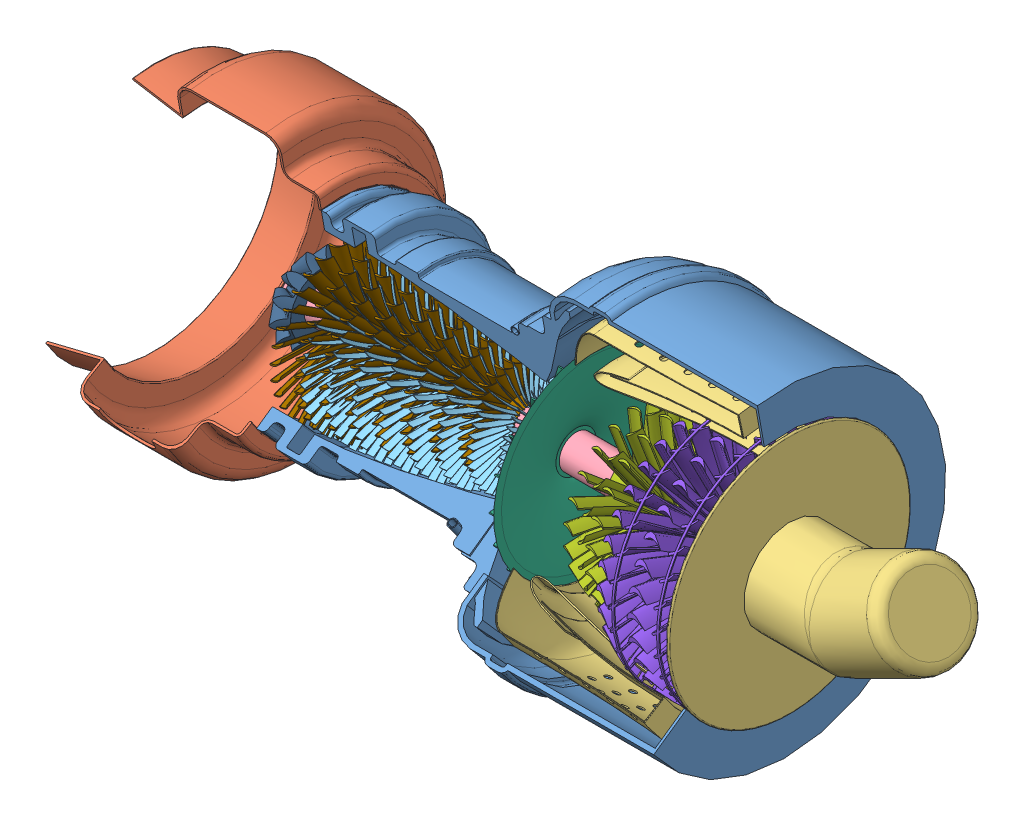
SolidWorks assembly Jet Gas Turbine Assembly, configuration Default. Lengths in mm.
Overall size (358.12 156.28 153.26).
10 component instances, 10 part files, 14 mates.
Components (placement in the parent):
- Compressor Housing-1: Compressor Housing [Default] at (41.278 135.5352 148.4921) size (198.89 147.12 133.82)
- Gear Housing-1: Gear Housing [Default] at (-33.532 135.5352 172.1021) size (82.19 132.5 124.3)
- F Housing-1: F Housing [Default] at (27.3575 135.5352 172.1021) x (1 0 0) z (0 -0.204596 0.978846) size (163.49 132.73 128.83)
- Shaft-1: Shaft [Default] at (157.6947 135.5352 172.1021) x (0 -0.328078 -0.94465) z (-1 0 0) size (15 15 210)
- Compressor Blade-1: Compressor Blade [Default] at (-16.2813 135.5352 172.1021) x (0 -0.28215 -0.95937) z (1 0 0) size (70.56 70.56 80)
- coplepe-3: coplepe [Default] at (79.1724 135.5352 172.1021) x (0 0.011714 0.999931) z (-1 0 0) size (95.21 95.21 17.99)
- compressor runner turbine-2: compressor runner turbine [Default] at (124.3085 135.5352 172.1021) x (0 0.195485 0.980707) z (-1 0 0) size (84.17 84.1 30)
- Drive Turbine-2: Drive Turbine [Default] at (156.7297 135.5352 172.1021) x (0 0.018348 0.999832) z (-1 0 0) size (106.71 106.71 85)
- Stator compressor-1: Stator compressor [Default] at (51.3243 135.5352 172.1021) x (0 -0.136427 0.99065) z (-1 0 0) size (72.35 72.38 80)
- straight bevel pinion_iso-1: straight bevel pinion_iso [ISO - Straight bevel pinion 2.75M12PT 12GT 20PA 12FW ---12O75H10MD15.0N] at (-41.4462 135.5352 172.1021) x (-1 0 0) z (0 -0.643855 -0.765147) size (12.56 36.5 36.5)
Mates (geometry in assembly coordinates):
- Coincident1: coincident: line of assembly; line of assembly; line of Compressor Housing-1 through (-39.9211 135.5352 172.1021) axis (1 0 0); line of Gear Housing-1 through (-33.532 135.5352 172.1021) axis (-1 0 0)
- Coincident2: coincident: plane of assembly; plane of assembly; plane of Compressor Housing-1 through (-33.532 179.5955 179.8711) normal (-1 0 0); plane of Gear Housing-1 through (-33.532 110.9602 214.6673) normal (1 0 0)
- Coincident3: coincident: line of assembly; line of assembly; line of Compressor Housing-1 through (-39.9211 135.5352 172.1021) axis (1 0 0); line of F Housing-1 through (-203.8591 135.5352 172.1021) axis (1 0 0)
- Distance3: distance = 7.5 mm: plane of assembly; plane of assembly; plane of F Housing-1 through (157.8575 106.8113 218.4183) normal (1 0 0); plane of Compressor Housing-1 through (165.3575 188.6064 181.46) normal (1 0 0)
- Concentric1: concentric: circle of assembly; circle of assembly; circle of Gear Housing-1; circle of Shaft-1
- Concentric2: concentric: circle of assembly; circle of assembly; circle of Gear Housing-1; circle of Shaft-1
- Concentric4: concentric: cylinder of ? through (-46.8 135.5352 172.1021) axis (1 0 0) radius 7.5; cylinder of Compressor Blade-1 through (63.7187 135.5352 172.1021) axis (-1 0 0) radius 7.2
- Coincident10: coincident: line of assembly; line of assembly; line of F Housing-1 through (-203.8591 135.5352 172.1021) axis (1 0 0); line of coplepe-3 through (32.2405 135.5352 172.1021) axis (1 0 0)
- Concentric5: concentric: cylinder of ? through (-46.8 135.5352 172.1021) axis (1 0 0) radius 7.5; cylinder of compressor runner turbine-2 through (94.3085 135.5352 172.1021) axis (1 0 0) radius 7.5
- Coincident12: coincident: plane of assembly; point of assembly; plane of Compressor Housing-1 through (23.1065 168.0396 177.8335) normal (0 -0.173648 0.984808); moEndPointRef_w of compressor runner turbine-2
- Concentric6: concentric: cylinder of ? through (-46.8 135.5352 172.1021) axis (1 0 0) radius 7.5; cylinder of Drive Turbine-2 through (186.7297 135.5352 172.1021) axis (-1 0 0) radius 6.5
- Concentric7: concentric: cylinder of ? through (-46.8 135.5352 172.1021) axis (1 0 0) radius 7.5; cylinder of Stator compressor-1 through (-28.6757 135.5352 172.1021) axis (1 0 0) radius 7.5
- Concentric8: concentric: cylinder of ? through (-46.8 135.5352 172.1021) axis (1 0 0) radius 7.5; cylinder of straight bevel pinion_iso-1 through (-60.8348 135.5352 172.1021) axis (1 0 0) radius 7.5
- Coincident13: coincident: circle of assembly; circle of assembly; circle of Shaft-1; circle of straight bevel pinion_iso-1
